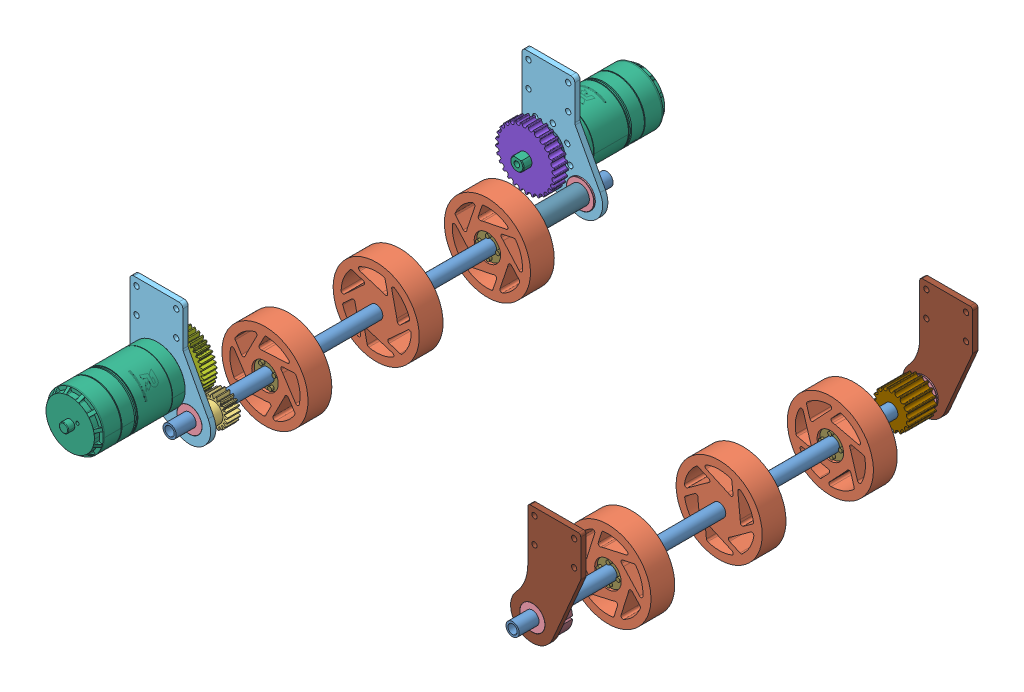
SolidWorks assembly 前后翻矿机构, configuration 默认. Lengths in mm.
Overall size (360.93 118.11 442.2).
30 component instances, 14 part files, 61 mates.
Components (placement in the parent):
- 10mm铝管-1: 10mm铝管 [默认] at (-129.5 0 0) x (1 0 0) z (0 0 -1) size (10 10 330)
- 10mm铝管-2: 10mm铝管 [默认] at (129.5 0 0) x (-1 0 0) z (0 0 -1) size (10 10 330)
- 翻矿打印件-1: 翻矿打印件 [默认] at (129.5 0 84) x (0.829736 0.558156 0) z (0 0 1) size (65 65 18)
- 翻矿打印件-2: 翻矿打印件 [默认] at (129.5 0 -84) x (0.990398 0.138246 0) z (0 0 1) size (65 65 18)
- 翻矿打印件-3: 翻矿打印件 [默认] at (-129.5 0 -84) x (-0.047381 0.998877 0) z (0 0 1) size (65 65 18)
- 翻矿打印件-4: 翻矿打印件 [默认] at (-129.5 0 84) x (0.911199 0.411966 0) z (0 0 1) size (65 65 18)
- 圆柱齿轮20×1-1: 圆柱齿轮20×1 [默认] at (-125.8171 0 126) x (-0.64056 -0.767908 0) z (0 0 1) size (21.83 21.83 18)
- 法兰轴承-1: 法兰轴承 [10*19*5-1] at (-129.5 0 145) x (0.582685 0.812698 0) z (0.812698 -0.582685 0) size (21 5 21)
- 翻矿电机安装板-2: 翻矿电机安装板 [后驱] at (-129.5 0 150) x (-1 0 0) z (0 0 -1) size (61 89 4)
- RoboMaster M3508直流无刷减速电机-1: RoboMaster M3508直流无刷减速电机 [默认] at (-162.6696 2.0988 236.441) x (-0.91084 0.412759 0) z (0 0 -1) size (42 42.01 98.4)
- 圆柱齿轮40×1-1: 圆柱齿轮40×1 [默认] at (-153.5 18 126) x (0.992313 -0.123751 0) z (0 0 1) size (41.92 41.92 20)
- 翻矿电机安装板-3: 翻矿电机安装板 [前驱] at (-129.5 0 -146) x (-1 0 0) z (0 0 -1) size (62.48 89 4)
- RoboMaster M3508直流无刷减速电机-2: RoboMaster M3508直流无刷减速电机 [默认] at (-161.5702 0.8682 -236.441) x (0.893896 -0.448274 0) z (0 0 1) size (42 42.01 98.4)
- 法兰轴承-2: 法兰轴承 [10*19*5-1] at (-129.5 0 -145) x (-0.831063 -0.556179 0) z (0.556179 -0.831063 0) size (21 5 21)
- 大带轮5mx29-1: 大带轮5mx29 [A] at (-154.98 18 -72.58) x (0 0 -1) z (0.816888 -0.576796 0) size (10 44.91 44.97)
- 小带轮5mx18-1: 小带轮5mx18 [默认] at (129.5 0 -121) x (0 0 -1) z (0.777037 -0.629455 0) size (21 27.19 27.51)
- 推力球轴承-1: 推力球轴承 [51100 10*24*9] at (-154.98 18 -148.08) x (-0.468033 -0.883711 0) z (-0.883711 0.468033 0) size (24 9 24)
- 翻矿前连接板-1: 翻矿前连接板 [默认] at (129.5 0 -150) size (53 89.5 4)
- 法兰轴承-3: 法兰轴承 [10*19*5-1] at (129.5 0 -145) x (-0.896596 -0.442849 0) z (0.442849 -0.896596 0) size (21 5 21)
- 翻矿前连接板-2: 翻矿前连接板 [默认] at (129.5 0 146) size (53 89.5 4)
- 法兰轴承-4: 法兰轴承 [10*19*5-1] at (129.5 0 145) x (0.110634 -0.993861 0) z (-0.993861 -0.110634 0) size (21 5 21)
- Z21-10-20-13-1: Z21-10-20-13 [默认] at (129.5 0 84.5) size (20 20 15)
- Z21-10-20-13-2: Z21-10-20-13 [默认] at (129.5 0 -83.5) x (0.99719 0.074916 0) z (0 0 1) size (20 20 15)
- Z21-10-20-13-3: Z21-10-20-13 [默认] at (-129.5 0 -83.5) x (0.999856 0.016974 0) z (0 0 1) size (20 20 15)
- Z21-10-20-13-4: Z21-10-20-13 [默认] at (-129.5 0 84.5) x (0.884281 0.466955 0) z (0 0 1) size (20 20 15)
- 翻矿打印件-5: 翻矿打印件 [默认] at (129.5 0 0) x (-0.967813 -0.251669 0) z (0 0 -1) size (65 65 18)
- 翻矿打印件-6: 翻矿打印件 [默认] at (-129.5 0 0) x (-0.931626 -0.363419 0) z (0 0 -1) size (65 65 18)
- Z21-10-20-13-5: Z21-10-20-13 [默认] at (-129.5 0 -0.5) x (-0.987188 -0.159561 0) z (0 0 -1) size (20 20 15)
- 紧固环-1: 紧固环 [默认] at (129.5 0 139.7) size (29.93 30 10)
- 限位打印件-1: 限位打印件 [默认] at (-129.5 0 -119) size (14 14 52)
Mates (geometry in assembly coordinates):
- 重合4: coincident aligned: plane of 10mm铝管-1 through (-129.5 0 0) normal (0 0 -1); plane of 10mm铝管-2 through (129.5 0 0) normal (0 0 -1)
- 对称3: symmetric aligned: plane of 翻矿打印件-1 through (129.5 0 75) normal (0 0 -1); plane of 翻矿打印件-2 through (129.5 0 -75) normal (0 0 1)
- 距离1: distance = 150 mm anti-aligned: plane of 翻矿打印件-2 through (129.5 0 -75) normal (0 0 1); plane of 翻矿打印件-1 through (129.5 0 75) normal (0 0 -1)
- 重合6: coincident aligned: plane of 翻矿打印件-1 through (129.5 0 75) normal (0 0 -1); plane of 翻矿打印件-4 through (-129.5 0 75) normal (0 0 -1)
- 重合7: coincident aligned: plane of 翻矿打印件-2 through (129.5 0 -75) normal (0 0 1); plane of 翻矿打印件-3 through (-129.5 0 -75) normal (0 0 1)
- 距离2: distance = 194 mm: cylinder of 翻矿打印件-3 through (-129.5 0 -75) axis (0 0 -1) radius 32.5; cylinder of 翻矿打印件-2 through (129.5 0 -75) axis (0 0 -1) radius 32.5
- 平行2: parallel anti-aligned: plane of 翻矿电机安装板-2 through (-174.5 73 146) normal (-1 0 0)
- 距离4: distance = 150 mm aligned: plane of 翻矿电机安装板-2 through (-153.5 18 150) normal (0 0 1)
- 同心12: concentric anti-aligned: cylinder of 法兰轴承-1 through (-129.5 0 150) axis (0 0 -1) radius 9.5; cylinder of 翻矿电机安装板-2 through (-129.5 0 146) axis (0 0 1) radius 9.5
- 重合11: coincident anti-aligned: plane of 法兰轴承-1 through (-129.5 0 146) normal (0 0 1); plane of 翻矿电机安装板-2 through (-153.5 18 146) normal (0 0 -1)
- 距离5: distance = 1 mm anti-aligned: plane of 圆柱齿轮20×1-1 through (-125.8171 0 144) normal (0 0 1); plane of 法兰轴承-1 through (-129.5 0 145) normal (0 0 -1)
- 同心13: concentric anti-aligned: cylinder of 翻矿电机安装板-2 through (-153.5 18 146) axis (0 0 1) radius 13.05; cylinder of RoboMaster M3508直流无刷减速电机-1 through (-153.5 18 130.8808) axis (0 0 -1) radius 21
- 重合13: coincident anti-aligned: plane of 翻矿电机安装板-2 through (-153.5 18 150) normal (0 0 1); plane of RoboMaster M3508直流无刷减速电机-1 through (-153.8674 5.0052 150) normal (0 0 -1)
- 同心14: concentric anti-aligned: cylinder of RoboMaster M3508直流无刷减速电机-1 through (-153.5 18 122.7) axis (0 0 -1) radius 5; cylinder of 圆柱齿轮40×1-1 through (-153.5 18 118) axis (0 0 1) radius 5
- 重合14: coincident aligned: plane of 圆柱齿轮20×1-1 through (-125.8171 0 126) normal (0 0 -1); plane of 圆柱齿轮40×1-1 through (-153.5 18 126) normal (0 0 -1)
- 齿轮配合1: gear = 40 : 20 mm: cylinder of 圆柱齿轮20×1-1 through (-125.8171 0 136) axis (0 0 -1) radius 11; cylinder of 圆柱齿轮40×1-1 through (-153.5 18 136) axis (0 0 -1) radius 21
- 对称4: symmetric aligned: plane of 翻矿电机安装板-2 through (-153.5 18 146) normal (0 0 -1); plane of 翻矿电机安装板-3 through (-153.5 18 -146) normal (0 0 1)
- 同心16: concentric aligned: cylinder of 翻矿电机安装板-3 through (-154.98 18 -86.603) axis (0 0 -1) radius 21; cylinder of RoboMaster M3508直流无刷减速电机-2 through (-154.98 18 -186) axis (0 0 -1) radius 21
- 重合16: coincident anti-aligned: plane of 翻矿电机安装板-3 through (-153.5 18 -150) normal (0 0 -1); plane of RoboMaster M3508直流无刷减速电机-2 through (-164.8493 9.5385 -150) normal (0 0 1)
- 重合17: coincident anti-aligned: plane of 翻矿电机安装板-3 through (-153.5 18 -146) normal (0 0 1); plane of 法兰轴承-2 through (-129.5 0 -146) normal (0 0 -1)
- 平行3: parallel aligned: plane of 翻矿电机安装板-2 through (-174.5 73 146) normal (-1 0 0); plane of 翻矿电机安装板-3 through (-174.5 73 -150) normal (-1 0 0)
- 同心21: concentric anti-aligned: cylinder of RoboMaster M3508直流无刷减速电机-2 through (-154.98 18 -122.7) axis (0 0 1) radius 5; cylinder of 大带轮5mx29-1 through (-154.98 18 -114.9379) axis (0 0 -1) radius 5
- 同心23: concentric anti-aligned: cylinder of RoboMaster M3508直流无刷减速电机-2 through (-154.98 18 -122.7) axis (0 0 1) radius 5; cylinder of 推力球轴承-1 through (-154.98 18 -139.08) axis (0 0 -1) radius 12
- 重合18: coincident anti-aligned: plane of RoboMaster M3508直流无刷减速电机-2 through (-154.98 18 -148.08) normal (0 0 1); plane of 推力球轴承-1 through (-154.98 18 -148.08) normal (0 0 -1)
- 重合19: coincident anti-aligned: plane of 大带轮5mx29-1 through (-154.98 18 -139.08) normal (0 0 -1); plane of 推力球轴承-1 through (-154.98 18 -139.08) normal (0 0 1)
- 重合20: coincident aligned: plane of 翻矿电机安装板-3 through (-153.5 18 -150) normal (0 0 -1); plane of 翻矿前连接板-1 through (129.5 0 -150) normal (0 0 -1)
- 平行4: parallel aligned: plane of 翻矿前连接板-1 through (129.5 0 -150) normal (1 0 0)
- 同心25: concentric anti-aligned: cylinder of 翻矿前连接板-1 through (129.5 0 -146) axis (0 0 -1) radius 9.5; cylinder of 法兰轴承-3 through (129.5 0 -150) axis (0 0 1) radius 9.5
- 重合21: coincident anti-aligned: plane of 翻矿前连接板-1 through (129.5 0 -146) normal (0 0 1); plane of 法兰轴承-3 through (129.5 0 -146) normal (0 0 -1)
- 距离6: distance = 3 mm anti-aligned: plane of 小带轮5mx18-1 through (129.5 0 -142) normal (0 0 -1); plane of 法兰轴承-3 through (129.5 0 -145) normal (0 0 1)
- 对称5: symmetric aligned: plane of 翻矿前连接板-1 through (129.5 0 -146) normal (0 0 1); plane of 翻矿前连接板-2 through (129.5 0 146) normal (0 0 -1)
- 平行5: parallel aligned: plane of 翻矿前连接板-1 through (126 43 -224.1485) normal (-1 0 0); plane of 翻矿前连接板-2 through (126 43 71.8515) normal (-1 0 0)
- 重合22: coincident anti-aligned: plane of 翻矿前连接板-2 through (129.5 0 146) normal (0 0 -1); plane of 法兰轴承-4 through (129.5 0 146) normal (0 0 1)
- 重合23: coincident anti-aligned: plane of 翻矿打印件-1 through (129.5 0 78) normal (0 0 1); plane of Z21-10-20-13-1 through (129.5 0 78) normal (0 0 -1)
- 重合24: coincident anti-aligned: plane of 翻矿打印件-2 through (129.5 0 -90) normal (0 0 1); plane of Z21-10-20-13-2 through (129.5 0 -90) normal (0 0 -1)
- 同心30: concentric anti-aligned: cylinder of 翻矿打印件-3 through (-129.5 0 -90) axis (0 0 1) radius 10; cylinder of Z21-10-20-13-3 through (-129.5 0 -77) axis (0 0 -1) radius 5
- 重合25: coincident anti-aligned: plane of 翻矿打印件-3 through (-129.5 0 -90) normal (0 0 1); plane of Z21-10-20-13-3 through (-129.5 0 -90) normal (0 0 -1)
- 同心32: concentric anti-aligned: cylinder of 翻矿打印件-4 through (-129.5 0 78) axis (0 0 1) radius 10; cylinder of Z21-10-20-13-4 through (-129.5 0 91) axis (0 0 -1) radius 10
- 重合26: coincident anti-aligned: plane of 翻矿打印件-4 through (-129.5 0 78) normal (0 0 1); plane of Z21-10-20-13-4 through (-129.5 0 78) normal (0 0 -1)
- 对称6: symmetric aligned: plane of 翻矿打印件-5 through (129.5 0 9) normal (0 0 1); plane of 翻矿打印件-5 through (129.5 0 -9) normal (0 0 -1)
- 重合27: coincident aligned: plane of 翻矿打印件-5 through (129.5 0 -9) normal (0 0 -1); plane of 翻矿打印件-6 through (-129.5 0 -9) normal (0 0 -1)
- 重合28: coincident anti-aligned: plane of 翻矿打印件-6 through (-129.5 0 6) normal (0 0 -1); plane of Z21-10-20-13-5 through (-129.5 0 6) normal (0 0 1)
- 同心33: concentric aligned: cylinder of 10mm铝管-1 through (-129.5 0 -165) axis (0 0 1) radius 5; cylinder of 翻矿打印件-6 through (-129.5 0 -9) axis (0 0 1) radius 5
- 同心34: concentric anti-aligned: cylinder of 10mm铝管-2 through (129.5 0 -165) axis (0 0 1) radius 5; cylinder of Z21-10-20-13-1 through (129.5 0 91) axis (0 0 -1) radius 5
- 重合29: coincident anti-aligned: plane of 10mm铝管-1 through (-129.5 0 0) normal (0 -1 0)
- 重合30: coincident anti-aligned: plane of 10mm铝管-1 through (-129.5 0 0) normal (0 -1 0); plane of 10mm铝管-2 through (129.5 0 0) normal (0 1 0)
- 重合31: coincident anti-aligned: plane of 10mm铝管-1 through (-129.5 0 0) normal (0 0 -1)
- 对称7: symmetric aligned: plane of 10mm铝管-1 through (-129.5 0 0) normal (1 0 0); plane of 10mm铝管-2 through (129.5 0 0) normal (-1 0 0)
- 同心35: concentric anti-aligned: cylinder of 10mm铝管-1 through (-129.5 0 -165) axis (0 0 1) radius 5; cylinder of Z21-10-20-13-4 through (-129.5 0 91) axis (0 0 -1) radius 5
- 同心36: concentric anti-aligned: cylinder of 10mm铝管-1 through (-129.5 0 -165) axis (0 0 1) radius 5; cylinder of 法兰轴承-1 through (-129.5 0 150) axis (0 0 -1) radius 5
- 同心37: concentric aligned: cylinder of 10mm铝管-2 through (129.5 0 -165) axis (0 0 1) radius 5; cylinder of 翻矿打印件-5 through (129.5 0 -9) axis (0 0 1) radius 5
- 同心38: concentric anti-aligned: cylinder of 翻矿打印件-1 through (129.5 0 78) axis (0 0 1) radius 10; cylinder of Z21-10-20-13-1 through (129.5 0 91) axis (0 0 -1) radius 10
- 同心39: concentric anti-aligned: cylinder of 10mm铝管-2 through (129.5 0 -165) axis (0 0 1) radius 5; cylinder of 翻矿打印件-2 through (129.5 0 -75) axis (0 0 -1) radius 32.5
- 同心40: concentric anti-aligned: cylinder of 10mm铝管-1 through (-129.5 0 -165) axis (0 0 1) radius 5; cylinder of Z21-10-20-13-3 through (-129.5 0 -77) axis (0 0 -1) radius 5
- 同心41: concentric anti-aligned: cylinder of 10mm铝管-2 through (129.5 0 -165) axis (0 0 1) radius 5; cylinder of 小带轮5mx18-1 through (129.5 0 -106.8579) axis (0 0 -1) radius 5
- 同心42: concentric aligned: cylinder of 10mm铝管-2 through (129.5 0 -165) axis (0 0 1) radius 5; cylinder of 法兰轴承-3 through (129.5 0 -150) axis (0 0 1) radius 5
- 同心43: concentric anti-aligned: cylinder of 10mm铝管-2 through (129.5 0 -165) axis (0 0 1) radius 5; cylinder of 翻矿前连接板-2 through (129.5 0 150) axis (0 0 -1) radius 9.5
- 同心44: concentric anti-aligned: cylinder of 10mm铝管-2 through (129.5 0 -165) axis (0 0 1) radius 5; cylinder of 紧固环-1 through (129.5 0 144.7) axis (0 0 -1) radius 5
- 距离7: distance = 0.3 mm anti-aligned: plane of 紧固环-1 through (129.5 0 144.7) normal (0 0 1); plane of 法兰轴承-4 through (129.5 0 145) normal (0 0 -1)
- 同心45: concentric anti-aligned: cylinder of 10mm铝管-1 through (-129.5 0 -165) axis (0 0 1) radius 5; cylinder of 限位打印件-1 through (-129.5 0 -93) axis (0 0 -1) radius 7
- 重合32: coincident anti-aligned: plane of 法兰轴承-2 through (-129.5 0 -145) normal (0 0 1); plane of 限位打印件-1 through (-129.5 0 -145) normal (0 0 -1)
